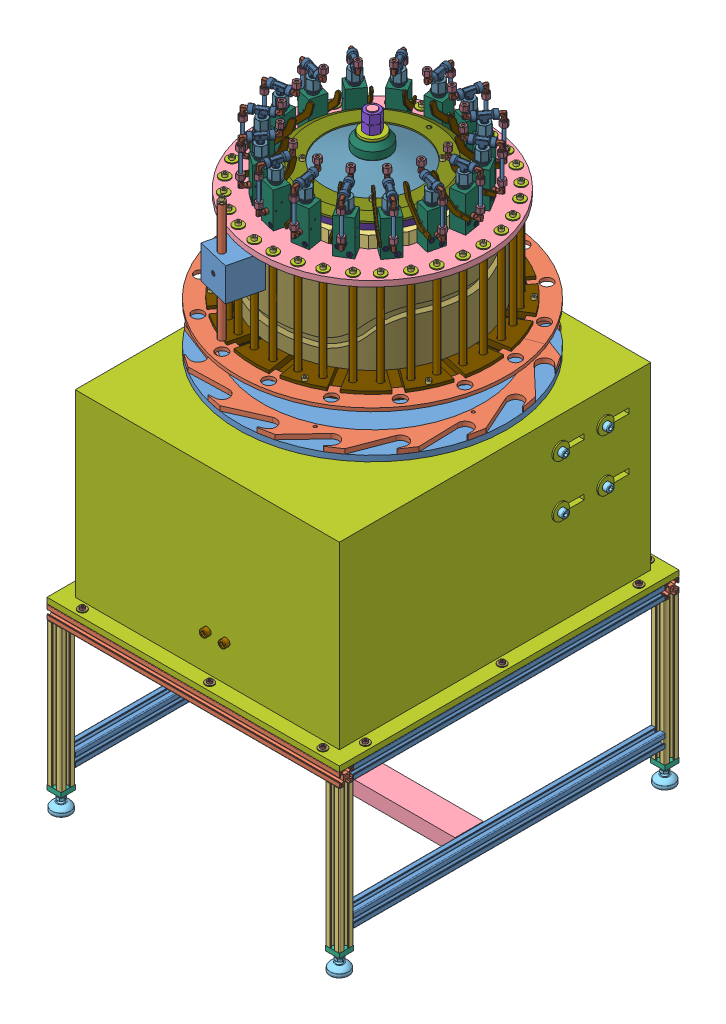
SolidWorks assembly Assieme_FINALE, configuration Default. Lengths in mm. (continued)
Components (placement in the parent): (continued)
- assieme parte rotante-2: assieme parte rotante [Default] at (-8.3038 623.9178 -528.0599) x (0 1 0) z (-0.913062 0 0.407822) size (749.63 778.63 778.63) (continued)
  - M6 16mm-39: M6 16mm [ISO 4762 M6 x 16 - 16N] at (167.0433 -190.119 494.6741) x (1 0 0) z (0 -0.991445 0.130526) size (22 10 10)
  - M6 16mm-40: M6 16mm [ISO 4762 M6 x 16 - 16N] at (167.0433 -143.7592 568.3922) x (1 0 0) z (0 -0.866025 0.5) size (22 10 10)
  - M6 16mm-41: M6 16mm [ISO 4762 M6 x 16 - 16N] at (167.0433 -72.7177 618.7576) x (1 0 0) z (0 -0.608761 0.793353) size (22 10 10)
  - M6 16mm-42: M6 16mm [ISO 4762 M6 x 16 - 16N] at (167.0433 12.1901 638.1029) x (1 0 0) z (0 -0.258819 0.965926) size (22 10 10)
  - M6 16mm-43: M6 16mm [ISO 4762 M6 x 16 - 16N] at (167.0433 98.0378 623.4827) x (1 0 0) z (0 0.130526 0.991445) size (22 10 10)
  - M6 16mm-44: M6 16mm [ISO 4762 M6 x 16 - 16N] at (167.0433 171.7559 577.1229) x (1 0 0) z (0 0.5 0.866025) size (22 10 10)
  - M6 16mm-45: M6 16mm [ISO 4762 M6 x 16 - 16N] at (167.0433 222.1213 506.0814) x (1 0 0) z (0 0.793353 0.608761) size (22 10 10)
  - M6 16mm-46: M6 16mm [ISO 4762 M6 x 16 - 16N] at (167.0433 241.4666 421.1736) x (1 0 0) z (0 0.965926 0.258819) size (22 10 10)
  - M6 16mm-47: M6 16mm [ISO 4762 M6 x 16 - 16N] at (167.0433 226.8464 335.3259) x (1 0 0) z (0 0.991445 -0.130526) size (22 10 10)
  - M6 16mm-48: M6 16mm [ISO 4762 M6 x 16 - 16N] at (167.0433 180.4866 261.6078) x (1 0 0) z (0 0.866025 -0.5) size (22 10 10)
  - M6 16mm-49: M6 16mm [ISO 4762 M6 x 16 - 16N] at (167.0433 109.4451 211.2424) x (1 0 0) z (0 0.608761 -0.793353) size (22 10 10)
  - asta scorrimento carello-18: asta scorrimento carello [Default] at (287.5433 -61.3104 206.5173) x (0 -0.130526 -0.991445) z (-1 0 0) size (12 12 225)
  - asta scorrimento carello-19: asta scorrimento carello [Default] at (287.5433 -135.0285 252.8771) x (0 -0.5 -0.866025) z (-1 0 0) size (12 12 225)
  - asta scorrimento carello-20: asta scorrimento carello [Default] at (287.5433 -185.3939 323.9186) x (0 -0.793353 -0.608761) z (-1 0 0) size (12 12 225)
  - asta scorrimento carello-21: asta scorrimento carello [Default] at (287.5433 -204.7392 408.8264) x (0 -0.965926 -0.258819) z (-1 0 0) size (12 12 225)
  - asta scorrimento carello-22: asta scorrimento carello [Default] at (287.5433 -190.119 494.6741) x (0 -0.991445 0.130526) z (-1 0 0) size (12 12 225)
  - asta scorrimento carello-23: asta scorrimento carello [Default] at (287.5433 -143.7592 568.3922) x (0 -0.866025 0.5) z (-1 0 0) size (12 12 225)
  - asta scorrimento carello-24: asta scorrimento carello [Default] at (287.5433 -72.7177 618.7576) x (0 -0.608761 0.793353) z (-1 0 0) size (12 12 225)
  - asta scorrimento carello-25: asta scorrimento carello [Default] at (287.5433 12.1901 638.1029) x (0 -0.258819 0.965926) z (-1 0 0) size (12 12 225)
  - asta scorrimento carello-26: asta scorrimento carello [Default] at (287.5433 98.0378 623.4827) x (0 0.130526 0.991445) z (-1 0 0) size (12 12 225)
  - asta scorrimento carello-27: asta scorrimento carello [Default] at (287.5433 171.7559 577.1229) x (0 0.5 0.866025) z (-1 0 0) size (12 12 225)
  - asta scorrimento carello-28: asta scorrimento carello [Default] at (287.5433 222.1213 506.0814) x (0 0.793353 0.608761) z (-1 0 0) size (12 12 225)
  - asta scorrimento carello-29: asta scorrimento carello [Default] at (287.5433 241.4666 421.1736) x (0 0.965926 0.258819) z (-1 0 0) size (12 12 225)
  - asta scorrimento carello-30: asta scorrimento carello [Default] at (287.5433 226.8464 335.3259) x (0 0.991445 -0.130526) z (-1 0 0) size (12 12 225)
  - asta scorrimento carello-31: asta scorrimento carello [Default] at (287.5433 180.4866 261.6078) x (0 0.866025 -0.5) z (-1 0 0) size (12 12 225)
  - asta scorrimento carello-32: asta scorrimento carello [Default] at (287.5433 109.4451 211.2424) x (0 0.608761 -0.793353) z (-1 0 0) size (12 12 225)
  - rondella M6-129: rondella M6 [Washer ISO 7094 - 6] at (400.0433 -61.3104 206.5173) x (-1 0 0) z (0 0.991445 -0.130526) size (2 22 22)
  - rondella M6-130: rondella M6 [Washer ISO 7094 - 6] at (400.0433 -135.0285 252.8771) x (-1 0 0) z (0 0.866025 -0.5) size (2 22 22)
  - rondella M6-131: rondella M6 [Washer ISO 7094 - 6] at (400.0433 -185.3939 323.9186) x (-1 0 0) z (0 0.608761 -0.793353) size (2 22 22)
  - rondella M6-132: rondella M6 [Washer ISO 7094 - 6] at (400.0433 -204.7392 408.8264) x (-1 0 0) z (0 0.258819 -0.965926) size (2 22 22)
  - rondella M6-133: rondella M6 [Washer ISO 7094 - 6] at (400.0433 -190.119 494.6741) x (-1 0 0) z (0 -0.130526 -0.991445) size (2 22 22)
  - rondella M6-134: rondella M6 [Washer ISO 7094 - 6] at (400.0433 -143.7592 568.3922) x (-1 0 0) z (0 -0.5 -0.866025) size (2 22 22)
  - rondella M6-135: rondella M6 [Washer ISO 7094 - 6] at (400.0433 -72.7177 618.7576) x (-1 0 0) z (0 -0.793353 -0.608761) size (2 22 22)
  - rondella M6-136: rondella M6 [Washer ISO 7094 - 6] at (400.0433 12.1901 638.1029) x (-1 0 0) z (0 -0.965926 -0.258819) size (2 22 22)
  - rondella M6-137: rondella M6 [Washer ISO 7094 - 6] at (400.0433 98.0378 623.4827) x (-1 0 0) z (0 -0.991445 0.130526) size (2 22 22)
  - rondella M6-138: rondella M6 [Washer ISO 7094 - 6] at (400.0433 171.7559 577.1229) x (-1 0 0) z (0 -0.866025 0.5) size (2 22 22)
  - rondella M6-139: rondella M6 [Washer ISO 7094 - 6] at (400.0433 222.1213 506.0814) x (-1 0 0) z (0 -0.608761 0.793353) size (2 22 22)
  - rondella M6-140: rondella M6 [Washer ISO 7094 - 6] at (400.0433 241.4666 421.1736) x (-1 0 0) z (0 -0.258819 0.965926) size (2 22 22)
  - rondella M6-141: rondella M6 [Washer ISO 7094 - 6] at (400.0433 226.8464 335.3259) x (-1 0 0) z (0 0.130526 0.991445) size (2 22 22)
  - rondella M6-142: rondella M6 [Washer ISO 7094 - 6] at (400.0433 180.4866 261.6078) x (-1 0 0) z (0 0.5 0.866025) size (2 22 22)
  - rondella M6-143: rondella M6 [Washer ISO 7094 - 6] at (400.0433 109.4451 211.2424) x (-1 0 0) z (0 0.793353 0.608761) size (2 22 22)
  - M6 16mm-50: M6 16mm [ISO 4762 M6 x 16 - 16N] at (408.0433 -61.3104 206.5173) x (-1 0 0) z (0 0.130526 0.991445) size (22 10 10)
  - M6 16mm-51: M6 16mm [ISO 4762 M6 x 16 - 16N] at (408.0433 -135.0285 252.8771) x (-1 0 0) z (0 0.5 0.866025) size (22 10 10)
  - M6 16mm-52: M6 16mm [ISO 4762 M6 x 16 - 16N] at (408.0433 -185.3939 323.9186) x (-1 0 0) z (0 0.793353 0.608761) size (22 10 10)
  - M6 16mm-53: M6 16mm [ISO 4762 M6 x 16 - 16N] at (408.0433 -204.7392 408.8264) x (-1 0 0) z (0 0.965926 0.258819) size (22 10 10)
  - M6 16mm-54: M6 16mm [ISO 4762 M6 x 16 - 16N] at (408.0433 -190.119 494.6741) x (-1 0 0) z (0 0.991445 -0.130526) size (22 10 10)
  - M6 16mm-55: M6 16mm [ISO 4762 M6 x 16 - 16N] at (408.0433 -143.7592 568.3922) x (-1 0 0) z (0 0.866025 -0.5) size (22 10 10)
  - M6 16mm-56: M6 16mm [ISO 4762 M6 x 16 - 16N] at (408.0433 -72.7177 618.7576) x (-1 0 0) z (0 0.608761 -0.793353) size (22 10 10)
  - M6 16mm-57: M6 16mm [ISO 4762 M6 x 16 - 16N] at (408.0433 12.1901 638.1029) x (-1 0 0) z (0 0.258819 -0.965926) size (22 10 10)
  - M6 16mm-58: M6 16mm [ISO 4762 M6 x 16 - 16N] at (408.0433 98.0378 623.4827) x (-1 0 0) z (0 -0.130526 -0.991445) size (22 10 10)
  - M6 16mm-59: M6 16mm [ISO 4762 M6 x 16 - 16N] at (408.0433 171.7559 577.1229) x (-1 0 0) z (0 -0.5 -0.866025) size (22 10 10)
  - M6 16mm-60: M6 16mm [ISO 4762 M6 x 16 - 16N] at (408.0433 222.1213 506.0814) x (-1 0 0) z (0 -0.793353 -0.608761) size (22 10 10)
  - M6 16mm-61: M6 16mm [ISO 4762 M6 x 16 - 16N] at (408.0433 241.4666 421.1736) x (-1 0 0) z (0 -0.965926 -0.258819) size (22 10 10)
  - M6 16mm-62: M6 16mm [ISO 4762 M6 x 16 - 16N] at (408.0433 226.8464 335.3259) x (-1 0 0) z (0 -0.991445 0.130526) size (22 10 10)
  - M6 16mm-63: M6 16mm [ISO 4762 M6 x 16 - 16N] at (408.0433 180.4866 261.6078) x (-1 0 0) z (0 -0.866025 0.5) size (22 10 10)
  - M6 16mm-64: M6 16mm [ISO 4762 M6 x 16 - 16N] at (408.0433 109.4451 211.2424) x (-1 0 0) z (0 -0.608761 0.793353) size (22 10 10)
  - AssiemeValvola-2: AssiemeValvola [Default] at (515.3257 40.5532 246.4544) x (0 -0.130526 0.991445) z (0 0.991445 0.130526) size (90.26 138.63 38)
    - RaccordoT-1: RaccordoT [Default] at origin size (43 29.75 16.5)
    - Raccordo a L-1: Raccordo a L [Default] at (-30 0 0) x (0 -1 0) z (0 0 -1) size (28.34 25.51 14.01)
      - 1809_06_10_01-1: 1809_06_10_01 [Default] at origin size (22.49 23 10)
      - 1809_06_10_02-1: 1809_06_10_02 [Default] at origin size (6.5 8.5 8.5)
      - 1809_06_10_03-1: 1809_06_10_03 [Default] at origin size (11.02 15.01 14.01)
    - Raccordo a L-2: Raccordo a L [Default] at (30 0 0) x (0 1 0) z (0 0 -1) size (28.34 25.51 14.01)
      - 1809_06_10_01-1: 1809_06_10_01 [Default] at origin size (22.49 23 10)
      - 1809_06_10_02-1: 1809_06_10_02 [Default] at origin size (6.5 8.5 8.5)
      - 1809_06_10_03-1: 1809_06_10_03 [Default] at origin size (11.02 15.01 14.01)
    - TappoChiusura-1: TappoChiusura [Default] at (0 -32 0) x (0 -1 0) z (0 0 1) size (38.28 26.74 26.74)
    - CorpoValvola-1: CorpoValvola [Default] at (-15 -115.2824 0) size (30 75 34)
    - Raccordo a L-3: Raccordo a L [Default] at (-30 -88.2824 0) x (0 1 0) z (0 0 1) size (28.34 25.51 14.01)
      - 1809_06_10_01-1: 1809_06_10_01 [Default] at origin size (22.49 23 10)
      - 1809_06_10_02-1: 1809_06_10_02 [Default] at origin size (6.5 8.5 8.5)
      - 1809_06_10_03-1: 1809_06_10_03 [Default] at origin size (11.02 15.01 14.01)
    - Spina_3x38-1: Spina_3x38 [Default] at (0 -68.2824 -21) x (-1 0 0) z (0 0 1) size (3 3 38)
    - Spina_3x38-2: Spina_3x38 [Default] at (-10 -80.2824 -21) x (0.996193 0.087174 0) z (0 0 1) size (3 3 38)
    - M5 40mm-3: M5 40mm [ISO 4762 M5 x 40 - 40N] at (-14.6 -108.7824 9) size (45 8.5 8.5)
    - M5 40mm-2: M5 40mm [ISO 4762 M5 x 40 - 40N] at (-14.6 -96.7824 -9) size (45 8.5 8.5)
    - LevaValvola-1: LevaValvola [Default] at (-24.507 -86.571 -17) x (0.996193 0.087174 0) z (0 0 1) size (77.55 60.2 4)
    - Tubo-1: Tubo [Default] at (-30 -15.9665 0) x (1 0 0) z (0 -1 0) size (6 6 56.4)
  - AssiemeValvola-3: AssiemeValvola [Default] at (515.3257 -25.6355 250.7926) x (0 0.258819 0.965926) z (0 0.965926 -0.258819) size (90.26 138.63 38)
    - RaccordoT-1: RaccordoT [Default] at origin size (43 29.75 16.5)
    - Raccordo a L-1: Raccordo a L [Default] at (-30 0 0) x (0 -1 0) z (0 0 -1) size (28.34 25.51 14.01)
      - 1809_06_10_01-1: 1809_06_10_01 [Default] at origin size (22.49 23 10)
      - 1809_06_10_02-1: 1809_06_10_02 [Default] at origin size (6.5 8.5 8.5)
      - 1809_06_10_03-1: 1809_06_10_03 [Default] at origin size (11.02 15.01 14.01)
    - Raccordo a L-2: Raccordo a L [Default] at (30 0 0) x (0 1 0) z (0 0 -1) size (28.34 25.51 14.01)
      - 1809_06_10_01-1: 1809_06_10_01 [Default] at origin size (22.49 23 10)
      - 1809_06_10_02-1: 1809_06_10_02 [Default] at origin size (6.5 8.5 8.5)
      - 1809_06_10_03-1: 1809_06_10_03 [Default] at origin size (11.02 15.01 14.01)
    - TappoChiusura-1: TappoChiusura [Default] at (0 -32 0) x (0 -1 0) z (0 0 1) size (38.28 26.74 26.74)
    - CorpoValvola-1: CorpoValvola [Default] at (-15 -115.2824 0) size (30 75 34)
    - Raccordo a L-3: Raccordo a L [Default] at (-30 -88.2824 0) x (0 1 0) z (0 0 1) size (28.34 25.51 14.01)
      - 1809_06_10_01-1: 1809_06_10_01 [Default] at origin size (22.49 23 10)
      - 1809_06_10_02-1: 1809_06_10_02 [Default] at origin size (6.5 8.5 8.5)
      - 1809_06_10_03-1: 1809_06_10_03 [Default] at origin size (11.02 15.01 14.01)
    - Spina_3x38-1: Spina_3x38 [Default] at (0 -68.2824 -21) x (-1 0 0) z (0 0 1) size (3 3 38)
    - Spina_3x38-2: Spina_3x38 [Default] at (-10 -80.2824 -21) x (0.996193 0.087174 0) z (0 0 1) size (3 3 38)
    - M5 40mm-3: M5 40mm [ISO 4762 M5 x 40 - 40N] at (-14.6 -108.7824 9) size (45 8.5 8.5)
    - M5 40mm-2: M5 40mm [ISO 4762 M5 x 40 - 40N] at (-14.6 -96.7824 -9) size (45 8.5 8.5)
    - LevaValvola-1: LevaValvola [Default] at (-24.507 -86.571 -17) x (0.996193 0.087174 0) z (0 0 1) size (77.55 60.2 4)
    - Tubo-1: Tubo [Default] at (-30 -15.9665 0) x (1 0 0) z (0 -1 0) size (6 6 56.4)
  - AssiemeValvola-4: AssiemeValvola [Default] at (515.3257 -85.1257 280.1299) x (0 0.608761 0.793353) z (0 0.793353 -0.608761) size (90.26 138.63 38)
    - RaccordoT-1: RaccordoT [Default] at origin size (43 29.75 16.5)
    - Raccordo a L-1: Raccordo a L [Default] at (-30 0 0) x (0 -1 0) z (0 0 -1) size (28.34 25.51 14.01)
      - 1809_06_10_01-1: 1809_06_10_01 [Default] at origin size (22.49 23 10)
      - 1809_06_10_02-1: 1809_06_10_02 [Default] at origin size (6.5 8.5 8.5)
      - 1809_06_10_03-1: 1809_06_10_03 [Default] at origin size (11.02 15.01 14.01)
    - Raccordo a L-2: Raccordo a L [Default] at (30 0 0) x (0 1 0) z (0 0 -1) size (28.34 25.51 14.01)
      - 1809_06_10_01-1: 1809_06_10_01 [Default] at origin size (22.49 23 10)
      - 1809_06_10_02-1: 1809_06_10_02 [Default] at origin size (6.5 8.5 8.5)
      - 1809_06_10_03-1: 1809_06_10_03 [Default] at origin size (11.02 15.01 14.01)
    - TappoChiusura-1: TappoChiusura [Default] at (0 -32 0) x (0 -1 0) z (0 0 1) size (38.28 26.74 26.74)
    - CorpoValvola-1: CorpoValvola [Default] at (-15 -115.2824 0) size (30 75 34)
    - Raccordo a L-3: Raccordo a L [Default] at (-30 -88.2824 0) x (0 1 0) z (0 0 1) size (28.34 25.51 14.01)
      - 1809_06_10_01-1: 1809_06_10_01 [Default] at origin size (22.49 23 10)
      - 1809_06_10_02-1: 1809_06_10_02 [Default] at origin size (6.5 8.5 8.5)
      - 1809_06_10_03-1: 1809_06_10_03 [Default] at origin size (11.02 15.01 14.01)
    - Spina_3x38-1: Spina_3x38 [Default] at (0 -68.2824 -21) x (-1 0 0) z (0 0 1) size (3 3 38)
    - Spina_3x38-2: Spina_3x38 [Default] at (-10 -80.2824 -21) x (0.996193 0.087174 0) z (0 0 1) size (3 3 38)
    - M5 40mm-3: M5 40mm [ISO 4762 M5 x 40 - 40N] at (-14.6 -108.7824 9) size (45 8.5 8.5)
    - M5 40mm-2: M5 40mm [ISO 4762 M5 x 40 - 40N] at (-14.6 -96.7824 -9) size (45 8.5 8.5)
    - LevaValvola-1: LevaValvola [Default] at (-24.507 -86.571 -17) x (0.996193 0.087174 0) z (0 0 1) size (77.55 60.2 4)
    - Tubo-1: Tubo [Default] at (-30 -15.9665 0) x (1 0 0) z (0 -1 0) size (6 6 56.4)
  - AssiemeValvola-5: AssiemeValvola [Default] at (515.3257 -128.8606 330) x (0 0.866025 0.5) z (0 0.5 -0.866025) size (90.26 138.63 38)
    - RaccordoT-1: RaccordoT [Default] at origin size (43 29.75 16.5)
    - Raccordo a L-1: Raccordo a L [Default] at (-30 0 0) x (0 -1 0) z (0 0 -1) size (28.34 25.51 14.01)
      - 1809_06_10_01-1: 1809_06_10_01 [Default] at origin size (22.49 23 10)
      - 1809_06_10_02-1: 1809_06_10_02 [Default] at origin size (6.5 8.5 8.5)
      - 1809_06_10_03-1: 1809_06_10_03 [Default] at origin size (11.02 15.01 14.01)
    - Raccordo a L-2: Raccordo a L [Default] at (30 0 0) x (0 1 0) z (0 0 -1) size (28.34 25.51 14.01)
      - 1809_06_10_01-1: 1809_06_10_01 [Default] at origin size (22.49 23 10)
      - 1809_06_10_02-1: 1809_06_10_02 [Default] at origin size (6.5 8.5 8.5)
      - 1809_06_10_03-1: 1809_06_10_03 [Default] at origin size (11.02 15.01 14.01)
    - TappoChiusura-1: TappoChiusura [Default] at (0 -32 0) x (0 -1 0) z (0 0 1) size (38.28 26.74 26.74)
    - CorpoValvola-1: CorpoValvola [Default] at (-15 -115.2824 0) size (30 75 34)
    - Raccordo a L-3: Raccordo a L [Default] at (-30 -88.2824 0) x (0 1 0) z (0 0 1) size (28.34 25.51 14.01)
      - 1809_06_10_01-1: 1809_06_10_01 [Default] at origin size (22.49 23 10)
      - 1809_06_10_02-1: 1809_06_10_02 [Default] at origin size (6.5 8.5 8.5)
      - 1809_06_10_03-1: 1809_06_10_03 [Default] at origin size (11.02 15.01 14.01)
    - Spina_3x38-1: Spina_3x38 [Default] at (0 -68.2824 -21) x (-1 0 0) z (0 0 1) size (3 3 38)
    - Spina_3x38-2: Spina_3x38 [Default] at (-10 -80.2824 -21) x (0.996193 0.087174 0) z (0 0 1) size (3 3 38)
    - M5 40mm-3: M5 40mm [ISO 4762 M5 x 40 - 40N] at (-14.6 -108.7824 9) size (45 8.5 8.5)
    - M5 40mm-2: M5 40mm [ISO 4762 M5 x 40 - 40N] at (-14.6 -96.7824 -9) size (45 8.5 8.5)
    - LevaValvola-1: LevaValvola [Default] at (-24.507 -86.571 -17) x (0.996193 0.087174 0) z (0 0 1) size (77.55 60.2 4)
    - Tubo-1: Tubo [Default] at (-30 -15.9665 0) x (1 0 0) z (0 -1 0) size (6 6 56.4)
  - AssiemeValvola-6: AssiemeValvola [Default] at (515.3257 -150.1819 392.8105) x (0 0.991445 0.130526) z (0 0.130526 -0.991445) size (90.26 138.63 38)
    - RaccordoT-1: RaccordoT [Default] at origin size (43 29.75 16.5)
    - Raccordo a L-1: Raccordo a L [Default] at (-30 0 0) x (0 -1 0) z (0 0 -1) size (28.34 25.51 14.01)
      - 1809_06_10_01-1: 1809_06_10_01 [Default] at origin size (22.49 23 10)
      - 1809_06_10_02-1: 1809_06_10_02 [Default] at origin size (6.5 8.5 8.5)
      - 1809_06_10_03-1: 1809_06_10_03 [Default] at origin size (11.02 15.01 14.01)
    - Raccordo a L-2: Raccordo a L [Default] at (30 0 0) x (0 1 0) z (0 0 -1) size (28.34 25.51 14.01)
      - 1809_06_10_01-1: 1809_06_10_01 [Default] at origin size (22.49 23 10)
      - 1809_06_10_02-1: 1809_06_10_02 [Default] at origin size (6.5 8.5 8.5)
      - 1809_06_10_03-1: 1809_06_10_03 [Default] at origin size (11.02 15.01 14.01)
    - TappoChiusura-1: TappoChiusura [Default] at (0 -32 0) x (0 -1 0) z (0 0 1) size (38.28 26.74 26.74)
    - CorpoValvola-1: CorpoValvola [Default] at (-15 -115.2824 0) size (30 75 34)
    - Raccordo a L-3: Raccordo a L [Default] at (-30 -88.2824 0) x (0 1 0) z (0 0 1) size (28.34 25.51 14.01)
      - 1809_06_10_01-1: 1809_06_10_01 [Default] at origin size (22.49 23 10)
      - 1809_06_10_02-1: 1809_06_10_02 [Default] at origin size (6.5 8.5 8.5)
      - 1809_06_10_03-1: 1809_06_10_03 [Default] at origin size (11.02 15.01 14.01)
    - Spina_3x38-1: Spina_3x38 [Default] at (0 -68.2824 -21) x (-1 0 0) z (0 0 1) size (3 3 38)
    - Spina_3x38-2: Spina_3x38 [Default] at (-10 -80.2824 -21) x (0.996193 0.087174 0) z (0 0 1) size (3 3 38)
    - M5 40mm-3: M5 40mm [ISO 4762 M5 x 40 - 40N] at (-14.6 -108.7824 9) size (45 8.5 8.5)
    - M5 40mm-2: M5 40mm [ISO 4762 M5 x 40 - 40N] at (-14.6 -96.7824 -9) size (45 8.5 8.5)
    - LevaValvola-1: LevaValvola [Default] at (-24.507 -86.571 -17) x (0.996193 0.087174 0) z (0 0 1) size (77.55 60.2 4)
    - Tubo-1: Tubo [Default] at (-30 -15.9665 0) x (1 0 0) z (0 -1 0) size (6 6 56.4)
  - AssiemeValvola-7: AssiemeValvola [Default] at (515.3257 -145.8437 458.9992) x (0 0.965926 -0.258819) z (0 -0.258819 -0.965926) size (90.26 138.63 38)
    - RaccordoT-1: RaccordoT [Default] at origin size (43 29.75 16.5)
    - Raccordo a L-1: Raccordo a L [Default] at (-30 0 0) x (0 -1 0) z (0 0 -1) size (28.34 25.51 14.01)
      - 1809_06_10_01-1: 1809_06_10_01 [Default] at origin size (22.49 23 10)
      - 1809_06_10_02-1: 1809_06_10_02 [Default] at origin size (6.5 8.5 8.5)
      - 1809_06_10_03-1: 1809_06_10_03 [Default] at origin size (11.02 15.01 14.01)
    - Raccordo a L-2: Raccordo a L [Default] at (30 0 0) x (0 1 0) z (0 0 -1) size (28.34 25.51 14.01)
      - 1809_06_10_01-1: 1809_06_10_01 [Default] at origin size (22.49 23 10)
      - 1809_06_10_02-1: 1809_06_10_02 [Default] at origin size (6.5 8.5 8.5)
      - 1809_06_10_03-1: 1809_06_10_03 [Default] at origin size (11.02 15.01 14.01)
    - TappoChiusura-1: TappoChiusura [Default] at (0 -32 0) x (0 -1 0) z (0 0 1) size (38.28 26.74 26.74)
    - CorpoValvola-1: CorpoValvola [Default] at (-15 -115.2824 0) size (30 75 34)
    - Raccordo a L-3: Raccordo a L [Default] at (-30 -88.2824 0) x (0 1 0) z (0 0 1) size (28.34 25.51 14.01)
      - 1809_06_10_01-1: 1809_06_10_01 [Default] at origin size (22.49 23 10)
      - 1809_06_10_02-1: 1809_06_10_02 [Default] at origin size (6.5 8.5 8.5)
      - 1809_06_10_03-1: 1809_06_10_03 [Default] at origin size (11.02 15.01 14.01)
    - Spina_3x38-1: Spina_3x38 [Default] at (0 -68.2824 -21) x (-1 0 0) z (0 0 1) size (3 3 38)
    - Spina_3x38-2: Spina_3x38 [Default] at (-10 -80.2824 -21) x (0.996193 0.087174 0) z (0 0 1) size (3 3 38)
    - M5 40mm-3: M5 40mm [ISO 4762 M5 x 40 - 40N] at (-14.6 -108.7824 9) size (45 8.5 8.5)
    - M5 40mm-2: M5 40mm [ISO 4762 M5 x 40 - 40N] at (-14.6 -96.7824 -9) size (45 8.5 8.5)
    - LevaValvola-1: LevaValvola [Default] at (-24.507 -86.571 -17) x (0.996193 0.087174 0) z (0 0 1) size (77.55 60.2 4)
    - Tubo-1: Tubo [Default] at (-30 -15.9665 0) x (1 0 0) z (0 -1 0) size (6 6 56.4)
  - AssiemeValvola-8: AssiemeValvola [Default] at (515.3257 -116.5064 518.4894) x (0 0.793353 -0.608761) z (0 -0.608761 -0.793353) size (90.26 138.63 38)
    - RaccordoT-1: RaccordoT [Default] at origin size (43 29.75 16.5)
    - Raccordo a L-1: Raccordo a L [Default] at (-30 0 0) x (0 -1 0) z (0 0 -1) size (28.34 25.51 14.01)
      - 1809_06_10_01-1: 1809_06_10_01 [Default] at origin size (22.49 23 10)
      - 1809_06_10_02-1: 1809_06_10_02 [Default] at origin size (6.5 8.5 8.5)
      - 1809_06_10_03-1: 1809_06_10_03 [Default] at origin size (11.02 15.01 14.01)
    - Raccordo a L-2: Raccordo a L [Default] at (30 0 0) x (0 1 0) z (0 0 -1) size (28.34 25.51 14.01)
      - 1809_06_10_01-1: 1809_06_10_01 [Default] at origin size (22.49 23 10)
      - 1809_06_10_02-1: 1809_06_10_02 [Default] at origin size (6.5 8.5 8.5)
      - 1809_06_10_03-1: 1809_06_10_03 [Default] at origin size (11.02 15.01 14.01)
    - TappoChiusura-1: TappoChiusura [Default] at (0 -32 0) x (0 -1 0) z (0 0 1) size (38.28 26.74 26.74)
    - CorpoValvola-1: CorpoValvola [Default] at (-15 -115.2824 0) size (30 75 34)
    - Raccordo a L-3: Raccordo a L [Default] at (-30 -88.2824 0) x (0 1 0) z (0 0 1) size (28.34 25.51 14.01)
      - 1809_06_10_01-1: 1809_06_10_01 [Default] at origin size (22.49 23 10)
      - 1809_06_10_02-1: 1809_06_10_02 [Default] at origin size (6.5 8.5 8.5)
      - 1809_06_10_03-1: 1809_06_10_03 [Default] at origin size (11.02 15.01 14.01)
    - Spina_3x38-1: Spina_3x38 [Default] at (0 -68.2824 -21) x (-1 0 0) z (0 0 1) size (3 3 38)
    - Spina_3x38-2: Spina_3x38 [Default] at (-10 -80.2824 -21) x (0.996193 0.087174 0) z (0 0 1) size (3 3 38)
    - M5 40mm-3: M5 40mm [ISO 4762 M5 x 40 - 40N] at (-14.6 -108.7824 9) size (45 8.5 8.5)
    - M5 40mm-2: M5 40mm [ISO 4762 M5 x 40 - 40N] at (-14.6 -96.7824 -9) size (45 8.5 8.5)
    - LevaValvola-1: LevaValvola [Default] at (-24.507 -86.571 -17) x (0.996193 0.087174 0) z (0 0 1) size (77.55 60.2 4)
    - Tubo-1: Tubo [Default] at (-30 -15.9665 0) x (1 0 0) z (0 -1 0) size (6 6 56.4)
  - AssiemeValvola-9: AssiemeValvola [Default] at (515.3257 -66.6363 562.2243) x (0 0.5 -0.866025) z (0 -0.866025 -0.5) size (90.26 138.63 38)
    - RaccordoT-1: RaccordoT [Default] at origin size (43 29.75 16.5)
    - Raccordo a L-1: Raccordo a L [Default] at (-30 0 0) x (0 -1 0) z (0 0 -1) size (28.34 25.51 14.01)
      - 1809_06_10_01-1: 1809_06_10_01 [Default] at origin size (22.49 23 10)
      - 1809_06_10_02-1: 1809_06_10_02 [Default] at origin size (6.5 8.5 8.5)
      - 1809_06_10_03-1: 1809_06_10_03 [Default] at origin size (11.02 15.01 14.01)
    - Raccordo a L-2: Raccordo a L [Default] at (30 0 0) x (0 1 0) z (0 0 -1) size (28.34 25.51 14.01)
      - 1809_06_10_01-1: 1809_06_10_01 [Default] at origin size (22.49 23 10)
      - 1809_06_10_02-1: 1809_06_10_02 [Default] at origin size (6.5 8.5 8.5)
      - 1809_06_10_03-1: 1809_06_10_03 [Default] at origin size (11.02 15.01 14.01)
    - TappoChiusura-1: TappoChiusura [Default] at (0 -32 0) x (0 -1 0) z (0 0 1) size (38.28 26.74 26.74)
    - CorpoValvola-1: CorpoValvola [Default] at (-15 -115.2824 0) size (30 75 34)
    - Raccordo a L-3: Raccordo a L [Default] at (-30 -88.2824 0) x (0 1 0) z (0 0 1) size (28.34 25.51 14.01)
      - 1809_06_10_01-1: 1809_06_10_01 [Default] at origin size (22.49 23 10)
      - 1809_06_10_02-1: 1809_06_10_02 [Default] at origin size (6.5 8.5 8.5)
      - 1809_06_10_03-1: 1809_06_10_03 [Default] at origin size (11.02 15.01 14.01)
    - Spina_3x38-1: Spina_3x38 [Default] at (0 -68.2824 -21) x (-1 0 0) z (0 0 1) size (3 3 38)
    - Spina_3x38-2: Spina_3x38 [Default] at (-10 -80.2824 -21) x (0.996193 0.087174 0) z (0 0 1) size (3 3 38)
    - M5 40mm-3: M5 40mm [ISO 4762 M5 x 40 - 40N] at (-14.6 -108.7824 9) size (45 8.5 8.5)
    - M5 40mm-2: M5 40mm [ISO 4762 M5 x 40 - 40N] at (-14.6 -96.7824 -9) size (45 8.5 8.5)
    - LevaValvola-1: LevaValvola [Default] at (-24.507 -86.571 -17) x (0.996193 0.087174 0) z (0 0 1) size (77.55 60.2 4)
    - Tubo-1: Tubo [Default] at (-30 -15.9665 0) x (1 0 0) z (0 -1 0) size (6 6 56.4)
  - AssiemeValvola-10: AssiemeValvola [Default] at (515.3257 -3.8258 583.5456) x (0 0.130526 -0.991445) z (0 -0.991445 -0.130526) size (90.26 138.63 38)
    - RaccordoT-1: RaccordoT [Default] at origin size (43 29.75 16.5)
    - Raccordo a L-1: Raccordo a L [Default] at (-30 0 0) x (0 -1 0) z (0 0 -1) size (28.34 25.51 14.01)
      - 1809_06_10_01-1: 1809_06_10_01 [Default] at origin size (22.49 23 10)
      - 1809_06_10_02-1: 1809_06_10_02 [Default] at origin size (6.5 8.5 8.5)
      - 1809_06_10_03-1: 1809_06_10_03 [Default] at origin size (11.02 15.01 14.01)
    - Raccordo a L-2: Raccordo a L [Default] at (30 0 0) x (0 1 0) z (0 0 -1) size (28.34 25.51 14.01)
      - 1809_06_10_01-1: 1809_06_10_01 [Default] at origin size (22.49 23 10)
      - 1809_06_10_02-1: 1809_06_10_02 [Default] at origin size (6.5 8.5 8.5)
      - 1809_06_10_03-1: 1809_06_10_03 [Default] at origin size (11.02 15.01 14.01)
    - TappoChiusura-1: TappoChiusura [Default] at (0 -32 0) x (0 -1 0) z (0 0 1) size (38.28 26.74 26.74)
    - CorpoValvola-1: CorpoValvola [Default] at (-15 -115.2824 0) size (30 75 34)
    - Raccordo a L-3: Raccordo a L [Default] at (-30 -88.2824 0) x (0 1 0) z (0 0 1) size (28.34 25.51 14.01)
      - 1809_06_10_01-1: 1809_06_10_01 [Default] at origin size (22.49 23 10)
      - 1809_06_10_02-1: 1809_06_10_02 [Default] at origin size (6.5 8.5 8.5)
      - 1809_06_10_03-1: 1809_06_10_03 [Default] at origin size (11.02 15.01 14.01)
    - Spina_3x38-1: Spina_3x38 [Default] at (0 -68.2824 -21) x (-1 0 0) z (0 0 1) size (3 3 38)
    - Spina_3x38-2: Spina_3x38 [Default] at (-10 -80.2824 -21) x (0.996193 0.087174 0) z (0 0 1) size (3 3 38)
    - M5 40mm-3: M5 40mm [ISO 4762 M5 x 40 - 40N] at (-14.6 -108.7824 9) size (45 8.5 8.5)
    - M5 40mm-2: M5 40mm [ISO 4762 M5 x 40 - 40N] at (-14.6 -96.7824 -9) size (45 8.5 8.5)
    - LevaValvola-1: LevaValvola [Default] at (-24.507 -86.571 -17) x (0.996193 0.087174 0) z (0 0 1) size (77.55 60.2 4)
    - Tubo-1: Tubo [Default] at (-30 -15.9665 0) x (1 0 0) z (0 -1 0) size (6 6 56.4)
  - AssiemeValvola-11: AssiemeValvola [Default] at (515.3257 62.3629 579.2074) x (0 -0.258819 -0.965926) z (0 -0.965926 0.258819) size (90.26 138.63 38)
    - RaccordoT-1: RaccordoT [Default] at origin size (43 29.75 16.5)
    - Raccordo a L-1: Raccordo a L [Default] at (-30 0 0) x (0 -1 0) z (0 0 -1) size (28.34 25.51 14.01)
      - 1809_06_10_01-1: 1809_06_10_01 [Default] at origin size (22.49 23 10)
      - 1809_06_10_02-1: 1809_06_10_02 [Default] at origin size (6.5 8.5 8.5)
      - 1809_06_10_03-1: 1809_06_10_03 [Default] at origin size (11.02 15.01 14.01)
    - Raccordo a L-2: Raccordo a L [Default] at (30 0 0) x (0 1 0) z (0 0 -1) size (28.34 25.51 14.01)
      - 1809_06_10_01-1: 1809_06_10_01 [Default] at origin size (22.49 23 10)
      - 1809_06_10_02-1: 1809_06_10_02 [Default] at origin size (6.5 8.5 8.5)
      - 1809_06_10_03-1: 1809_06_10_03 [Default] at origin size (11.02 15.01 14.01)
    - TappoChiusura-1: TappoChiusura [Default] at (0 -32 0) x (0 -1 0) z (0 0 1) size (38.28 26.74 26.74)
    - CorpoValvola-1: CorpoValvola [Default] at (-15 -115.2824 0) size (30 75 34)
    - Raccordo a L-3: Raccordo a L [Default] at (-30 -88.2824 0) x (0 1 0) z (0 0 1) size (28.34 25.51 14.01)
      - 1809_06_10_01-1: 1809_06_10_01 [Default] at origin size (22.49 23 10)
      - 1809_06_10_02-1: 1809_06_10_02 [Default] at origin size (6.5 8.5 8.5)
      - 1809_06_10_03-1: 1809_06_10_03 [Default] at origin size (11.02 15.01 14.01)
    - Spina_3x38-1: Spina_3x38 [Default] at (0 -68.2824 -21) x (-1 0 0) z (0 0 1) size (3 3 38)
    - Spina_3x38-2: Spina_3x38 [Default] at (-10 -80.2824 -21) x (0.996193 0.087174 0) z (0 0 1) size (3 3 38)
    - M5 40mm-3: M5 40mm [ISO 4762 M5 x 40 - 40N] at (-14.6 -108.7824 9) size (45 8.5 8.5)
    - M5 40mm-2: M5 40mm [ISO 4762 M5 x 40 - 40N] at (-14.6 -96.7824 -9) size (45 8.5 8.5)
    - LevaValvola-1: LevaValvola [Default] at (-24.507 -86.571 -17) x (0.996193 0.087174 0) z (0 0 1) size (77.55 60.2 4)
    - Tubo-1: Tubo [Default] at (-30 -15.9665 0) x (1 0 0) z (0 -1 0) size (6 6 56.4)
  - AssiemeValvola-12: AssiemeValvola [Default] at (515.3257 121.8531 549.8701) x (0 -0.608761 -0.793353) z (0 -0.793353 0.608761) size (90.26 138.63 38)
    - RaccordoT-1: RaccordoT [Default] at origin size (43 29.75 16.5)
    - Raccordo a L-1: Raccordo a L [Default] at (-30 0 0) x (0 -1 0) z (0 0 -1) size (28.34 25.51 14.01)
      - 1809_06_10_01-1: 1809_06_10_01 [Default] at origin size (22.49 23 10)
      - 1809_06_10_02-1: 1809_06_10_02 [Default] at origin size (6.5 8.5 8.5)
      - 1809_06_10_03-1: 1809_06_10_03 [Default] at origin size (11.02 15.01 14.01)
    - Raccordo a L-2: Raccordo a L [Default] at (30 0 0) x (0 1 0) z (0 0 -1) size (28.34 25.51 14.01)
      - 1809_06_10_01-1: 1809_06_10_01 [Default] at origin size (22.49 23 10)
      - 1809_06_10_02-1: 1809_06_10_02 [Default] at origin size (6.5 8.5 8.5)
      - 1809_06_10_03-1: 1809_06_10_03 [Default] at origin size (11.02 15.01 14.01)
    - TappoChiusura-1: TappoChiusura [Default] at (0 -32 0) x (0 -1 0) z (0 0 1) size (38.28 26.74 26.74)
    - CorpoValvola-1: CorpoValvola [Default] at (-15 -115.2824 0) size (30 75 34)
    - Raccordo a L-3: Raccordo a L [Default] at (-30 -88.2824 0) x (0 1 0) z (0 0 1) size (28.34 25.51 14.01)
      - 1809_06_10_01-1: 1809_06_10_01 [Default] at origin size (22.49 23 10)
      - 1809_06_10_02-1: 1809_06_10_02 [Default] at origin size (6.5 8.5 8.5)
      - 1809_06_10_03-1: 1809_06_10_03 [Default] at origin size (11.02 15.01 14.01)
    - Spina_3x38-1: Spina_3x38 [Default] at (0 -68.2824 -21) x (-1 0 0) z (0 0 1) size (3 3 38)
    - Spina_3x38-2: Spina_3x38 [Default] at (-10 -80.2824 -21) x (0.996193 0.087174 0) z (0 0 1) size (3 3 38)
    - M5 40mm-3: M5 40mm [ISO 4762 M5 x 40 - 40N] at (-14.6 -108.7824 9) size (45 8.5 8.5)
    - M5 40mm-2: M5 40mm [ISO 4762 M5 x 40 - 40N] at (-14.6 -96.7824 -9) size (45 8.5 8.5)
    - LevaValvola-1: LevaValvola [Default] at (-24.507 -86.571 -17) x (0.996193 0.087174 0) z (0 0 1) size (77.55 60.2 4)
    - Tubo-1: Tubo [Default] at (-30 -15.9665 0) x (1 0 0) z (0 -1 0) size (6 6 56.4)
  - AssiemeValvola-13: AssiemeValvola [Default] at (515.3257 165.588 500) x (0 -0.866025 -0.5) z (0 -0.5 0.866025) size (90.26 138.63 38)
    - RaccordoT-1: RaccordoT [Default] at origin size (43 29.75 16.5)
    - Raccordo a L-1: Raccordo a L [Default] at (-30 0 0) x (0 -1 0) z (0 0 -1) size (28.34 25.51 14.01)
      - 1809_06_10_01-1: 1809_06_10_01 [Default] at origin size (22.49 23 10)
      - 1809_06_10_02-1: 1809_06_10_02 [Default] at origin size (6.5 8.5 8.5)
      - 1809_06_10_03-1: 1809_06_10_03 [Default] at origin size (11.02 15.01 14.01)
    - Raccordo a L-2: Raccordo a L [Default] at (30 0 0) x (0 1 0) z (0 0 -1) size (28.34 25.51 14.01)
      - 1809_06_10_01-1: 1809_06_10_01 [Default] at origin size (22.49 23 10)
      - 1809_06_10_02-1: 1809_06_10_02 [Default] at origin size (6.5 8.5 8.5)
      - 1809_06_10_03-1: 1809_06_10_03 [Default] at origin size (11.02 15.01 14.01)
    - TappoChiusura-1: TappoChiusura [Default] at (0 -32 0) x (0 -1 0) z (0 0 1) size (38.28 26.74 26.74)
    - CorpoValvola-1: CorpoValvola [Default] at (-15 -115.2824 0) size (30 75 34)
    - Raccordo a L-3: Raccordo a L [Default] at (-30 -88.2824 0) x (0 1 0) z (0 0 1) size (28.34 25.51 14.01)
      - 1809_06_10_01-1: 1809_06_10_01 [Default] at origin size (22.49 23 10)
      - 1809_06_10_02-1: 1809_06_10_02 [Default] at origin size (6.5 8.5 8.5)
      - 1809_06_10_03-1: 1809_06_10_03 [Default] at origin size (11.02 15.01 14.01)
    - Spina_3x38-1: Spina_3x38 [Default] at (0 -68.2824 -21) x (-1 0 0) z (0 0 1) size (3 3 38)
    - Spina_3x38-2: Spina_3x38 [Default] at (-10 -80.2824 -21) x (0.996193 0.087174 0) z (0 0 1) size (3 3 38)
    - M5 40mm-3: M5 40mm [ISO 4762 M5 x 40 - 40N] at (-14.6 -108.7824 9) size (45 8.5 8.5)
    - M5 40mm-2: M5 40mm [ISO 4762 M5 x 40 - 40N] at (-14.6 -96.7824 -9) size (45 8.5 8.5)
    - LevaValvola-1: LevaValvola [Default] at (-24.507 -86.571 -17) x (0.996193 0.087174 0) z (0 0 1) size (77.55 60.2 4)
    - Tubo-1: Tubo [Default] at (-30 -15.9665 0) x (1 0 0) z (0 -1 0) size (6 6 56.4)
  - AssiemeValvola-14: AssiemeValvola [Default] at (515.3257 186.9093 437.1895) x (0 -0.991445 -0.130526) z (0 -0.130526 0.991445) size (90.26 138.63 38)
    - RaccordoT-1: RaccordoT [Default] at origin size (43 29.75 16.5)
    - Raccordo a L-1: Raccordo a L [Default] at (-30 0 0) x (0 -1 0) z (0 0 -1) size (28.34 25.51 14.01)
      - 1809_06_10_01-1: 1809_06_10_01 [Default] at origin size (22.49 23 10)
      - 1809_06_10_02-1: 1809_06_10_02 [Default] at origin size (6.5 8.5 8.5)
      - 1809_06_10_03-1: 1809_06_10_03 [Default] at origin size (11.02 15.01 14.01)
    - Raccordo a L-2: Raccordo a L [Default] at (30 0 0) x (0 1 0) z (0 0 -1) size (28.34 25.51 14.01)
      - 1809_06_10_01-1: 1809_06_10_01 [Default] at origin size (22.49 23 10)
      - 1809_06_10_02-1: 1809_06_10_02 [Default] at origin size (6.5 8.5 8.5)
      - 1809_06_10_03-1: 1809_06_10_03 [Default] at origin size (11.02 15.01 14.01)
    - TappoChiusura-1: TappoChiusura [Default] at (0 -32 0) x (0 -1 0) z (0 0 1) size (38.28 26.74 26.74)
    - CorpoValvola-1: CorpoValvola [Default] at (-15 -115.2824 0) size (30 75 34)
    - Raccordo a L-3: Raccordo a L [Default] at (-30 -88.2824 0) x (0 1 0) z (0 0 1) size (28.34 25.51 14.01)
      - 1809_06_10_01-1: 1809_06_10_01 [Default] at origin size (22.49 23 10)
      - 1809_06_10_02-1: 1809_06_10_02 [Default] at origin size (6.5 8.5 8.5)
      - 1809_06_10_03-1: 1809_06_10_03 [Default] at origin size (11.02 15.01 14.01)
    - Spina_3x38-1: Spina_3x38 [Default] at (0 -68.2824 -21) x (-1 0 0) z (0 0 1) size (3 3 38)
    - Spina_3x38-2: Spina_3x38 [Default] at (-10 -80.2824 -21) x (0.996193 0.087174 0) z (0 0 1) size (3 3 38)
    - M5 40mm-3: M5 40mm [ISO 4762 M5 x 40 - 40N] at (-14.6 -108.7824 9) size (45 8.5 8.5)
    - M5 40mm-2: M5 40mm [ISO 4762 M5 x 40 - 40N] at (-14.6 -96.7824 -9) size (45 8.5 8.5)
